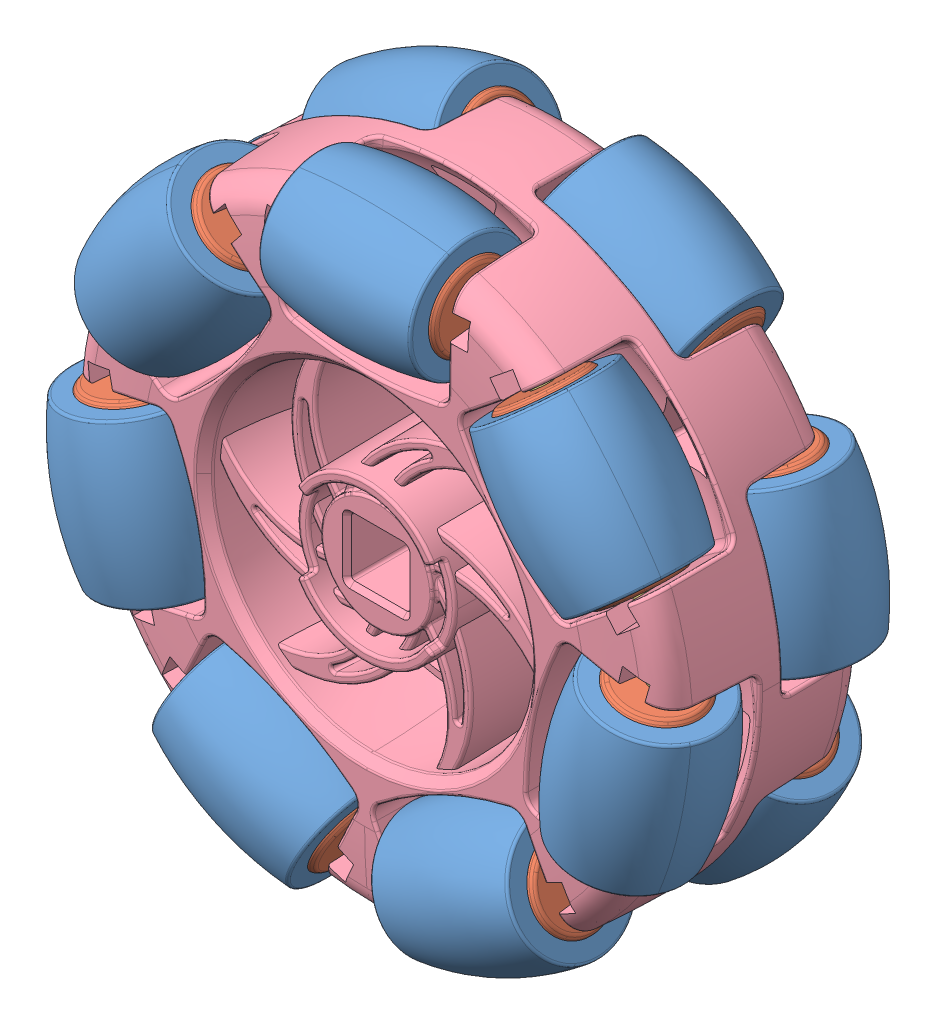
SolidWorks assembly 2.75 Omni-Directional Wheel - Double Roller (276-1902) , configuration Default. Lengths in mm.
Overall size (87.15 87.98 47.75).
58 component instances, 4 part files, 0 mates.
Components (placement in the parent):
- 2.75 Omni-Directional Wheel - Double Roller (276-1902) .step-1: 2.75 Omni-Directional Wheel - Double Roller (276-1902) .step [Default] at origin size (87.15 87.98 47.75)
  - 276-1902-010 Rev1.step-1: 276-1902-010 Rev1.step [Default] at (0 27.5 8) x (1 0 0) z (0 0.828233 0.560383) size (23 27.81 20.35)
    - 276-1902-011 Rev1.step-1: 276-1902-011 Rev1.step [Default] at (0 -6.325 -26.7627) x (1 0 0) z (0 -0.973191 0.23) size (16.5 15 25.03)
    - 276-1902-012 Rev1.step-1: 276-1902-012 Rev1.step [Default] at origin size (17.5 10.34 18.34)
    - 276-1902-003 Rev1.step-1: 276-1902-003 Rev1.step [Default] x (0 -0.928523 0.371275) z (1 0 0) size (2 2 23)
  - 276-1902-010 Rev1.step-2: 276-1902-010 Rev1.step [Default] at (0 -27.5 -8) x (1 0 0) z (0 0.410464 0.911877) size (23 27.81 20.35)
    - 276-1902-011 Rev1.step-1: 276-1902-011 Rev1.step [Default] at (0 -6.325 -26.7627) x (1 0 0) z (0 -0.973191 0.23) size (16.5 15 25.03)
    - 276-1902-012 Rev1.step-1: 276-1902-012 Rev1.step [Default] at origin size (17.5 10.34 18.34)
    - 276-1902-003 Rev1.step-1: 276-1902-003 Rev1.step [Default] x (0 -0.928523 0.371275) z (1 0 0) size (2 2 23)
  - 276-1902-010 Rev1.step-3: 276-1902-010 Rev1.step [Default] at (-21.5004 -17.146 -8) x (0.62349 -0.781831 0) z (0.320913 0.25592 0.911877) size (23 27.81 20.35)
    - 276-1902-011 Rev1.step-1: 276-1902-011 Rev1.step [Default] at (0 -6.325 -26.7627) x (1 0 0) z (0 -0.973191 0.23) size (16.5 15 25.03)
    - 276-1902-012 Rev1.step-1: 276-1902-012 Rev1.step [Default] at origin size (17.5 10.34 18.34)
    - 276-1902-003 Rev1.step-1: 276-1902-003 Rev1.step [Default] x (0 -0.928523 0.371275) z (1 0 0) size (2 2 23)
  - 276-1902-010 Rev1.step-4: 276-1902-010 Rev1.step [Default] at (-26.8105 6.1193 -8) x (-0.222521 -0.974928 0) z (0.400172 -0.091337 0.911877) size (23 27.81 20.35)
    - 276-1902-011 Rev1.step-1: 276-1902-011 Rev1.step [Default] at (0 -6.325 -26.7627) x (1 0 0) z (0 -0.973191 0.23) size (16.5 15 25.03)
    - 276-1902-012 Rev1.step-1: 276-1902-012 Rev1.step [Default] at origin size (17.5 10.34 18.34)
    - 276-1902-003 Rev1.step-1: 276-1902-003 Rev1.step [Default] x (0 -0.928523 0.371275) z (1 0 0) size (2 2 23)
  - 276-1902-010 Rev1.step-5: 276-1902-010 Rev1.step [Default] at (-11.9318 24.7766 -8) x (-0.900969 -0.433884 0) z (0.178093 -0.369815 0.911877) size (23 27.81 20.35)
    - 276-1902-011 Rev1.step-1: 276-1902-011 Rev1.step [Default] at (0 -6.325 -26.7627) x (1 0 0) z (0 -0.973191 0.23) size (16.5 15 25.03)
    - 276-1902-012 Rev1.step-1: 276-1902-012 Rev1.step [Default] at origin size (17.5 10.34 18.34)
    - 276-1902-003 Rev1.step-1: 276-1902-003 Rev1.step [Default] x (0 -0.928523 0.371275) z (1 0 0) size (2 2 23)
  - 276-1902-010 Rev1.step-6: 276-1902-010 Rev1.step [Default] at (11.9318 24.7766 -8) x (-0.900969 0.433884 0) z (-0.178093 -0.369815 0.911877) size (23 27.81 20.35)
    - 276-1902-011 Rev1.step-1: 276-1902-011 Rev1.step [Default] at (0 -6.325 -26.7627) x (1 0 0) z (0 -0.973191 0.23) size (16.5 15 25.03)
    - 276-1902-012 Rev1.step-1: 276-1902-012 Rev1.step [Default] at origin size (17.5 10.34 18.34)
    - 276-1902-003 Rev1.step-1: 276-1902-003 Rev1.step [Default] x (0 -0.928523 0.371275) z (1 0 0) size (2 2 23)
  - 276-1902-010 Rev1.step-7: 276-1902-010 Rev1.step [Default] at (26.8105 6.1193 -8) x (-0.222521 0.974928 0) z (-0.400172 -0.091337 0.911877) size (23 27.81 20.35)
    - 276-1902-011 Rev1.step-1: 276-1902-011 Rev1.step [Default] at (0 -6.325 -26.7627) x (1 0 0) z (0 -0.973191 0.23) size (16.5 15 25.03)
    - 276-1902-012 Rev1.step-1: 276-1902-012 Rev1.step [Default] at origin size (17.5 10.34 18.34)
    - 276-1902-003 Rev1.step-1: 276-1902-003 Rev1.step [Default] x (0 -0.928523 0.371275) z (1 0 0) size (2 2 23)
  - 276-1902-010 Rev1.step-8: 276-1902-010 Rev1.step [Default] at (21.5004 -17.146 -8) x (0.62349 0.781831 0) z (-0.320913 0.25592 0.911877) size (23 27.81 20.35)
    - 276-1902-011 Rev1.step-1: 276-1902-011 Rev1.step [Default] at (0 -6.325 -26.7627) x (1 0 0) z (0 -0.973191 0.23) size (16.5 15 25.03)
    - 276-1902-012 Rev1.step-1: 276-1902-012 Rev1.step [Default] at origin size (17.5 10.34 18.34)
    - 276-1902-003 Rev1.step-1: 276-1902-003 Rev1.step [Default] x (0 -0.928523 0.371275) z (1 0 0) size (2 2 23)
  - 276-1902-010 Rev1.step-9: 276-1902-010 Rev1.step [Default] at (21.5004 17.146 8) x (0.62349 -0.781831 0) z (0.647539 0.516395 0.560383) size (23 27.81 20.35)
    - 276-1902-011 Rev1.step-1: 276-1902-011 Rev1.step [Default] at (0 -6.325 -26.7627) x (1 0 0) z (0 -0.973191 0.23) size (16.5 15 25.03)
    - 276-1902-012 Rev1.step-1: 276-1902-012 Rev1.step [Default] at origin size (17.5 10.34 18.34)
    - 276-1902-003 Rev1.step-1: 276-1902-003 Rev1.step [Default] x (0 -0.928523 0.371275) z (1 0 0) size (2 2 23)
  - 276-1902-010 Rev1.step-10: 276-1902-010 Rev1.step [Default] at (26.8105 -6.1193 8) x (-0.222521 -0.974928 0) z (0.807468 -0.184299 0.560383) size (23 27.81 20.35)
    - 276-1902-011 Rev1.step-1: 276-1902-011 Rev1.step [Default] at (0 -6.325 -26.7627) x (1 0 0) z (0 -0.973191 0.23) size (16.5 15 25.03)
    - 276-1902-012 Rev1.step-1: 276-1902-012 Rev1.step [Default] at origin size (17.5 10.34 18.34)
    - 276-1902-003 Rev1.step-1: 276-1902-003 Rev1.step [Default] x (0 -0.928523 0.371275) z (1 0 0) size (2 2 23)
  - 276-1902-010 Rev1.step-11: 276-1902-010 Rev1.step [Default] at (11.9318 -24.7766 8) x (-0.900969 -0.433884 0) z (0.359357 -0.746212 0.560383) size (23 27.81 20.35)
    - 276-1902-011 Rev1.step-1: 276-1902-011 Rev1.step [Default] at (0 -6.325 -26.7627) x (1 0 0) z (0 -0.973191 0.23) size (16.5 15 25.03)
    - 276-1902-012 Rev1.step-1: 276-1902-012 Rev1.step [Default] at origin size (17.5 10.34 18.34)
    - 276-1902-003 Rev1.step-1: 276-1902-003 Rev1.step [Default] x (0 -0.928523 0.371275) z (1 0 0) size (2 2 23)
  - 276-1902-010 Rev1.step-12: 276-1902-010 Rev1.step [Default] at (-11.9318 -24.7766 8) x (-0.900969 0.433884 0) z (-0.359357 -0.746212 0.560383) size (23 27.81 20.35)
    - 276-1902-011 Rev1.step-1: 276-1902-011 Rev1.step [Default] at (0 -6.325 -26.7627) x (1 0 0) z (0 -0.973191 0.23) size (16.5 15 25.03)
    - 276-1902-012 Rev1.step-1: 276-1902-012 Rev1.step [Default] at origin size (17.5 10.34 18.34)
    - 276-1902-003 Rev1.step-1: 276-1902-003 Rev1.step [Default] x (0 -0.928523 0.371275) z (1 0 0) size (2 2 23)
  - 276-1902-010 Rev1.step-13: 276-1902-010 Rev1.step [Default] at (-26.8105 -6.1193 8) x (-0.222521 0.974928 0) z (-0.807468 -0.184299 0.560383) size (23 27.81 20.35)
    - 276-1902-011 Rev1.step-1: 276-1902-011 Rev1.step [Default] at (0 -6.325 -26.7627) x (1 0 0) z (0 -0.973191 0.23) size (16.5 15 25.03)
    - 276-1902-012 Rev1.step-1: 276-1902-012 Rev1.step [Default] at origin size (17.5 10.34 18.34)
    - 276-1902-003 Rev1.step-1: 276-1902-003 Rev1.step [Default] x (0 -0.928523 0.371275) z (1 0 0) size (2 2 23)
  - 276-1902-010 Rev1.step-14: 276-1902-010 Rev1.step [Default] at (-21.5004 17.146 8) x (0.62349 0.781831 0) z (-0.647539 0.516395 0.560383) size (23 27.81 20.35)
    - 276-1902-011 Rev1.step-1: 276-1902-011 Rev1.step [Default] at (0 -6.325 -26.7627) x (1 0 0) z (0 -0.973191 0.23) size (16.5 15 25.03)
    - 276-1902-012 Rev1.step-1: 276-1902-012 Rev1.step [Default] at origin size (17.5 10.34 18.34)
    - 276-1902-003 Rev1.step-1: 276-1902-003 Rev1.step [Default] x (0 -0.928523 0.371275) z (1 0 0) size (2 2 23)
  - 276-1902-002 Rev3.step-1: 276-1902-002 Rev3.step [Default] at origin size (66.55 66.02 25.07)
